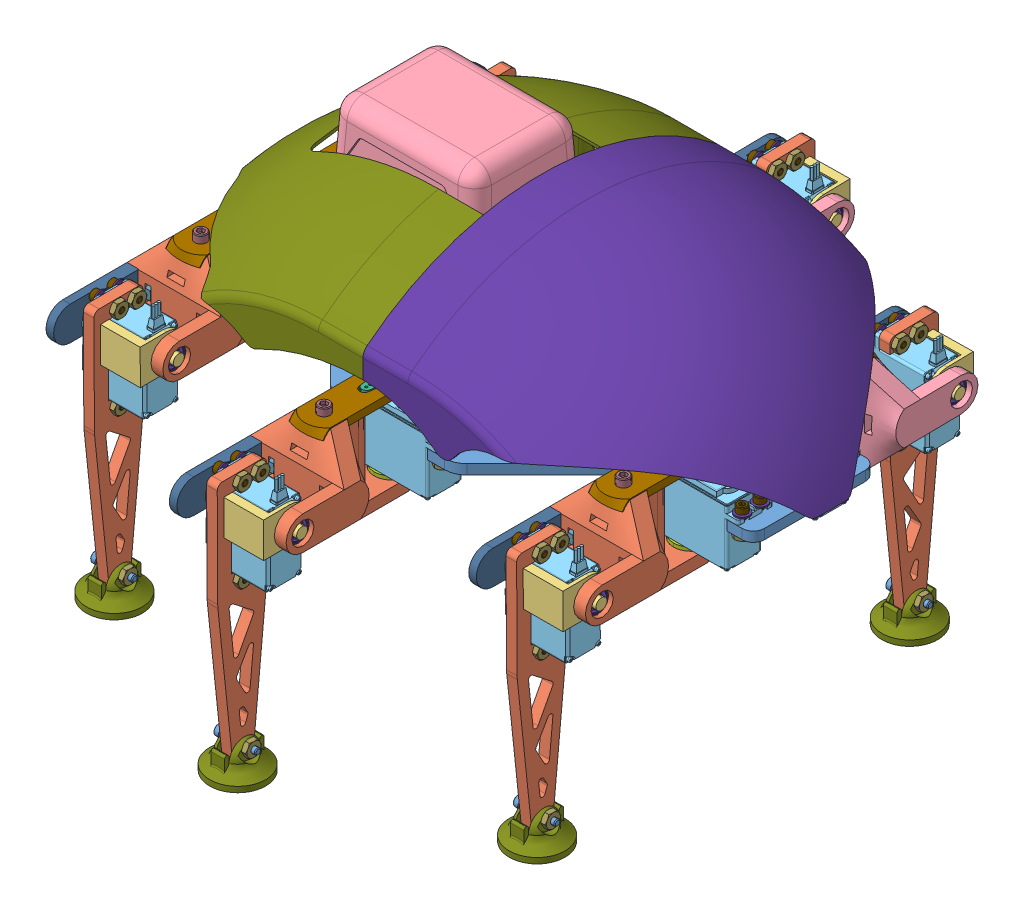
SolidWorks assembly Hexapod, configuration Défaut. Lengths in mm.
Overall size (338.69 233.7 350.77).
393 component instances, 35 part files, 155 mates.
Components (placement in the parent):
- Body_(Small)-5: Body_(Small) [Default] at (-310 -5.6 15) x (1 0 0) z (0 1 0) size (310 170 5.6)
- Leg_(Straight_Foot)-6: Leg_(Straight_Foot) [Default] at (-54.94 -26.67 -0.094) size (71.21 162.26 125.97) (flexible)
  - Foot_(Straight)-1: Foot_(Straight) [Default] at (4.9357 4.6704 -91.3697) x (0.014203 -0.004273 0.99989) z (-0.999899 0 0.014203) size (28 145.4 6)
  - bearing_mount_foot-1: bearing_mount_foot [Default] at (4.8169 16.6442 -99.7278) x (-0.014203 0.004273 -0.99989) z (0.999899 0 -0.014203) size (25 20 29.5)
  - Joint-1: Joint [Défaut] at (35.768 26.4662 -54.7315) x (-0.014203 0 -0.999899) z (0 1 0) size (96.52 53.26 53.26)
  - hs-422-2: hs-422 [Défaut] at (5.1023 6.612 -77.4562) x (-0.014203 0.004273 -0.99989) z (0.000061 0.999991 0.004272) size (19.81 42.09 58.23)
  - hs-422-3: hs-422 [Défaut] at (19.939 20.701 -19.812) x (0 0 1) z (-1 0 0) size (19.81 42.09 58.23)
  - hs-422_horn_straight-1: hs-422_horn_straight [Default] at (-16.9088 16.9412 -87.0065) x (0.014203 0 0.999899) z (0 1 0) size (33.93 4.93 8.79)
  - hs-422_horn_straight-2: hs-422_horn_straight [Default] at (9.652 42.5743 -9.906) x (-0.014203 0 -0.999899) z (-0.999899 0 0.014203) size (33.93 4.93 8.79)
  - Bearing_mount_leg-1: Bearing_mount_leg [Default] at (9.652 21 2.594) x (0 0 1) z (0 -1 0) size (35 20 30)
  - Bearing-1: Bearing [Default] at (9.652 -6.7498 -9.906) x (0.84763 0 0.530588) z (-0.530588 0 0.84763) size (13.87 4.75 13.87)
  - Bearing-2: Bearing [Default] at (32.2403 16.9412 -87.7047) x (0.007588 -0.845349 0.534161) z (-0.012007 -0.534214 -0.845264) size (13.87 4.75 13.87)
  - Joint_attachment_leg-1: Joint_attachment_leg [Défaut] at (35.768 26.4662 -54.7315) x (-0.014203 0 -0.999899) z (0 1 0) size (74.32 19.07 4.32)
  - Joint_attachment_foot-1: Joint_attachment_foot [Défaut] at (35.768 26.4662 -54.7315) x (-0.014203 0 -0.999899) z (0 1 0) size (64.08 6.7 19.07)
  - SBHCSCREW 0.112-40x0.25-HX-N-2: SBHCSCREW 0.112-40x0.25-HX-N [SBHCSCREW 0.112-40x0.25-HX-N] at (-19.9057 16.9412 -86.964) x (0.999899 0 -0.014203) z (-0.007102 0.866025 -0.49995) size (7.85 5.41 5.41)
  - SBHCSCREW 0.112-40x0.25-HX-N-3: SBHCSCREW 0.112-40x0.25-HX-N [SBHCSCREW 0.112-40x0.25-HX-N] at (9.652 45.5715 -9.906) x (0 -1 0) z (0.87304 0 0.487649) size (7.85 5.41 5.41)
  - MSHXNUT 0.138-32-D-N-15: MSHXNUT 0.138-32-D-N [MSHXNUT 0.138-32-D-N] at (5.0634 -17.1179 -82.3793) x (0.012331 0.496295 0.868066) z (-0.999899 0 0.014203) size (7.92 9.15 2.9)
  - MSHXNUT 0.138-32-D-N-16: MSHXNUT 0.138-32-D-N [MSHXNUT 0.138-32-D-N] at (4.9191 -17.0756 -92.5381) x (-0.01227 0.503696 -0.863794) z (-0.999899 0 0.014203) size (7.92 9.15 2.9)
  - MSHXNUT 0.138-32-D-N-17: MSHXNUT 0.138-32-D-N [MSHXNUT 0.138-32-D-N] at (5.0662 30.3817 -82.1827) x (0.000061 0.999991 0.004272) z (-0.999899 0 0.014203) size (7.92 9.15 2.9)
  - MSHXNUT 0.138-32-D-N-18: MSHXNUT 0.138-32-D-N [MSHXNUT 0.138-32-D-N] at (4.9219 30.4239 -92.3416) x (0.000061 0.999991 0.004272) z (-0.999899 0 0.014203) size (7.92 9.15 2.9)
  - HX-SHCS 0.164-32x0.5x0.5-N-1: HX-SHCS 0.164-32x0.5x0.5-N [HX-SHCS 0.164-32x0.5x0.5-N] at (9.1052 47.8568 -48.4) x (0 -1 0) z (0.014203 0 0.999899) size (16.87 6.86 6.86)
  - HX-SHCS 0.164-32x0.5x0.5-N-2: HX-SHCS 0.164-32x0.5x0.5-N [HX-SHCS 0.164-32x0.5x0.5-N] at (-21.967 16.9412 -59.205) x (0.999899 0 -0.014203) z (0.014203 0 0.999899) size (16.87 6.86 6.86)
  - MSHXNUT 0.164-32-D-N-11: MSHXNUT 0.164-32-D-N [MSHXNUT 0.164-32-D-N] at (9.1052 33.127 -48.4) x (0.87304 0 0.487649) z (0 1 0) size (8.74 10.09 3.3)
  - MSHXNUT 0.164-32-D-N-12: MSHXNUT 0.164-32-D-N [MSHXNUT 0.164-32-D-N] at (-7.2387 16.9412 -59.4142) x (0.014203 0 0.999899) z (-0.999899 0 0.014203) size (8.74 10.09 3.3)
  - HX-SHCS 0.112-40x0.5x0.5-N-7: HX-SHCS 0.112-40x0.5x0.5-N [HX-SHCS 0.112-40x0.5x0.5-N] at (-4.0273 11.7063 -99.6232) x (0.999899 0 -0.014203) z (0.014203 -0.004273 0.99989) size (15.54 4.65 4.65)
  - HX-SHCS 0.112-40x0.5x0.5-N-8: HX-SHCS 0.112-40x0.5x0.5-N [HX-SHCS 0.112-40x0.5x0.5-N] at (-4.0267 21.7062 -99.5805) x (0.999899 0 -0.014203) z (-0.014203 0.004273 -0.99989) size (15.54 4.65 4.65)
  - Slipper-1: Slipper [Default] at (1.9296 -111.2294 -91.7731) x (0.999899 0 -0.014203) z (0.014203 0 0.999899) size (35.48 18.25 37.71)
  - Narrow FW 0.138-1: Narrow FW 0.138 [Narrow FW 0.138] at (-3.4475 30.3814 -82.0597) x (0.999899 0 -0.014203) z (0.014203 0 0.999899) size (0.81 7.92 7.92)
  - HX-SHCS 0.138-32x0.5x0.5-N-2: HX-SHCS 0.138-32x0.5x0.5-N [HX-SHCS 0.138-32x0.5x0.5-N] at (-8.0191 30.3814 -81.9948) x (0.999899 0 -0.014203) z (0.014203 0 0.999899) size (16.21 5.74 5.74)
  - Narrow FW 0.138-2: Narrow FW 0.138 [Narrow FW 0.138] at (-3.4504 -17.1182 -82.2627) x (0.999899 0 -0.014203) z (0.014203 0 0.999899) size (0.81 7.92 7.92)
  - Narrow FW 0.138-3: Narrow FW 0.138 [Narrow FW 0.138] at (-3.5919 30.4248 -92.2186) x (0.999899 0 -0.014203) z (0.014203 0 0.999899) size (0.81 7.92 7.92)
  - Narrow FW 0.138-4: Narrow FW 0.138 [Narrow FW 0.138] at (-3.5947 -17.0748 -92.4216) x (0.999899 0 -0.014203) z (0.014203 0 0.999899) size (0.81 7.92 7.92)
  - HX-SHCS 0.138-32x0.5x0.5-N-3: HX-SHCS 0.138-32x0.5x0.5-N [HX-SHCS 0.138-32x0.5x0.5-N] at (-8.022 -17.1182 -82.1977) x (0.999899 0 -0.014203) z (0.014203 0 0.999899) size (16.21 5.74 5.74)
  - HX-SHCS 0.138-32x0.5x0.5-N-4: HX-SHCS 0.138-32x0.5x0.5-N [HX-SHCS 0.138-32x0.5x0.5-N] at (-8.1634 30.4248 -92.1537) x (0.999899 0 -0.014203) z (0.014203 0 0.999899) size (16.21 5.74 5.74)
  - HX-SHCS 0.138-32x0.5x0.5-N-5: HX-SHCS 0.138-32x0.5x0.5-N [HX-SHCS 0.138-32x0.5x0.5-N] at (-8.1663 -17.0748 -92.3566) x (0.999899 0 -0.014203) z (0.014203 0 0.999899) size (16.21 5.74 5.74)
  - HX-SHCS 0.138-32x0.5x0.5-N-6: HX-SHCS 0.138-32x0.5x0.5-N [HX-SHCS 0.138-32x0.5x0.5-N] at (-3.81 33.7566 -14.986) x (0 -1 0) z (-0.55878 0 0.829316) size (16.21 5.74 5.74)
  - Narrow FW 0.138-5: Narrow FW 0.138 [Narrow FW 0.138] at (-3.81 29.1846 -14.986) x (0 -1 0) z (0.55878 0 -0.829316) size (0.81 7.92 7.92)
  - Narrow FW 0.138-6: Narrow FW 0.138 [Narrow FW 0.138] at (43.69 29.1846 -14.986) x (0 -1 0) z (0.55878 0 -0.829316) size (0.81 7.92 7.92)
  - Narrow FW 0.138-7: Narrow FW 0.138 [Narrow FW 0.138] at (-3.81 29.1846 -4.826) x (0 -1 0) z (0.55878 0 -0.829316) size (0.81 7.92 7.92)
  - Narrow FW 0.138-8: Narrow FW 0.138 [Narrow FW 0.138] at (43.69 29.1846 -4.826) x (0 -1 0) z (0.55878 0 -0.829316) size (0.81 7.92 7.92)
  - HX-SHCS 0.138-32x0.5x0.5-N-7: HX-SHCS 0.138-32x0.5x0.5-N [HX-SHCS 0.138-32x0.5x0.5-N] at (43.69 33.7566 -14.986) x (0 -1 0) z (-0.55878 0 0.829316) size (16.21 5.74 5.74)
  - HX-SHCS 0.138-32x0.5x0.5-N-8: HX-SHCS 0.138-32x0.5x0.5-N [HX-SHCS 0.138-32x0.5x0.5-N] at (-3.81 33.7566 -4.826) x (0 -1 0) z (-0.55878 0 0.829316) size (16.21 5.74 5.74)
  - HX-SHCS 0.138-32x0.5x0.5-N-9: HX-SHCS 0.138-32x0.5x0.5-N [HX-SHCS 0.138-32x0.5x0.5-N] at (43.69 33.7566 -4.826) x (0 -1 0) z (-0.55878 0 0.829316) size (16.21 5.74 5.74)
  - HX-SHCS 0.138-32x0.75x0.75-N-10: HX-SHCS 0.138-32x0.75x0.75-N [HX-SHCS 0.138-32x0.75x0.75-N] at (-8.9913 -99.7294 -91.618) x (0.999899 0 -0.014203) z (-0.012539 -0.46966 -0.882758) size (22.56 5.74 5.74)
  - Narrow FW 0.138-10: Narrow FW 0.138 [Narrow FW 0.138] at (-5.2324 -99.7294 -91.6714) x (-0.999899 0 0.014203) z (-0.011665 -0.570502 -0.821213) size (0.81 7.92 7.92)
  - MSHXNUT 0.138-32-D-N-19: MSHXNUT 0.138-32-D-N [MSHXNUT 0.138-32-D-N] at (8.279 -99.7294 -91.8633) x (0 1 0) z (-0.999899 0 0.014203) size (7.92 9.15 2.9)
- Leg_(Straight_Foot)-7: Leg_(Straight_Foot) [Default] at (-294.94 -26.67 -0.094) size (71.21 162.26 125.97) (flexible)
  - Foot_(Straight)-1: Foot_(Straight) [Default] at (4.9357 4.6704 -91.3697) x (0.014203 -0.004273 0.99989) z (-0.999899 0 0.014203) size (28 145.4 6)
  - bearing_mount_foot-1: bearing_mount_foot [Default] at (4.8169 16.6442 -99.7278) x (-0.014203 0.004273 -0.99989) z (0.999899 0 -0.014203) size (25 20 29.5)
  - Joint-1: Joint [Défaut] at (35.768 26.4662 -54.7315) x (-0.014203 0 -0.999899) z (0 1 0) size (96.52 53.26 53.26)
  - hs-422-2: hs-422 [Défaut] at (5.1023 6.612 -77.4562) x (-0.014203 0.004273 -0.99989) z (0.000061 0.999991 0.004272) size (19.81 42.09 58.23)
  - hs-422-3: hs-422 [Défaut] at (19.939 20.701 -19.812) x (0 0 1) z (-1 0 0) size (19.81 42.09 58.23)
  - hs-422_horn_straight-1: hs-422_horn_straight [Default] at (-16.9088 16.9412 -87.0065) x (0.014203 0 0.999899) z (0 1 0) size (33.93 4.93 8.79)
  - hs-422_horn_straight-2: hs-422_horn_straight [Default] at (9.652 42.5743 -9.906) x (-0.014203 0 -0.999899) z (-0.999899 0 0.014203) size (33.93 4.93 8.79)
  - Bearing_mount_leg-1: Bearing_mount_leg [Default] at (9.652 21 2.594) x (0 0 1) z (0 -1 0) size (35 20 30)
  - Bearing-1: Bearing [Default] at (9.652 -6.7498 -9.906) x (0.84763 0 0.530588) z (-0.530588 0 0.84763) size (13.87 4.75 13.87)
  - Bearing-2: Bearing [Default] at (32.2403 16.9412 -87.7047) x (0.007588 -0.845349 0.534161) z (-0.012007 -0.534214 -0.845264) size (13.87 4.75 13.87)
  - Joint_attachment_leg-1: Joint_attachment_leg [Défaut] at (35.768 26.4662 -54.7315) x (-0.014203 0 -0.999899) z (0 1 0) size (74.32 19.07 4.32)
  - Joint_attachment_foot-1: Joint_attachment_foot [Défaut] at (35.768 26.4662 -54.7315) x (-0.014203 0 -0.999899) z (0 1 0) size (64.08 6.7 19.07)
  - SBHCSCREW 0.112-40x0.25-HX-N-2: SBHCSCREW 0.112-40x0.25-HX-N [SBHCSCREW 0.112-40x0.25-HX-N] at (-19.9057 16.9412 -86.964) x (0.999899 0 -0.014203) z (-0.007102 0.866025 -0.49995) size (7.85 5.41 5.41)
  - SBHCSCREW 0.112-40x0.25-HX-N-3: SBHCSCREW 0.112-40x0.25-HX-N [SBHCSCREW 0.112-40x0.25-HX-N] at (9.652 45.5715 -9.906) x (0 -1 0) z (0.87304 0 0.487649) size (7.85 5.41 5.41)
  - MSHXNUT 0.138-32-D-N-15: MSHXNUT 0.138-32-D-N [MSHXNUT 0.138-32-D-N] at (5.0634 -17.1179 -82.3793) x (0.012331 0.496295 0.868066) z (-0.999899 0 0.014203) size (7.92 9.15 2.9)
  - MSHXNUT 0.138-32-D-N-16: MSHXNUT 0.138-32-D-N [MSHXNUT 0.138-32-D-N] at (4.9191 -17.0756 -92.5381) x (-0.01227 0.503696 -0.863794) z (-0.999899 0 0.014203) size (7.92 9.15 2.9)
  - MSHXNUT 0.138-32-D-N-17: MSHXNUT 0.138-32-D-N [MSHXNUT 0.138-32-D-N] at (5.0662 30.3817 -82.1827) x (0.000061 0.999991 0.004272) z (-0.999899 0 0.014203) size (7.92 9.15 2.9)
  - MSHXNUT 0.138-32-D-N-18: MSHXNUT 0.138-32-D-N [MSHXNUT 0.138-32-D-N] at (4.9219 30.4239 -92.3416) x (0.000061 0.999991 0.004272) z (-0.999899 0 0.014203) size (7.92 9.15 2.9)
  - HX-SHCS 0.164-32x0.5x0.5-N-1: HX-SHCS 0.164-32x0.5x0.5-N [HX-SHCS 0.164-32x0.5x0.5-N] at (9.1052 47.8568 -48.4) x (0 -1 0) z (0.014203 0 0.999899) size (16.87 6.86 6.86)
  - HX-SHCS 0.164-32x0.5x0.5-N-2: HX-SHCS 0.164-32x0.5x0.5-N [HX-SHCS 0.164-32x0.5x0.5-N] at (-21.967 16.9412 -59.205) x (0.999899 0 -0.014203) z (0.014203 0 0.999899) size (16.87 6.86 6.86)
  - MSHXNUT 0.164-32-D-N-11: MSHXNUT 0.164-32-D-N [MSHXNUT 0.164-32-D-N] at (9.1052 33.127 -48.4) x (0.87304 0 0.487649) z (0 1 0) size (8.74 10.09 3.3)
  - MSHXNUT 0.164-32-D-N-12: MSHXNUT 0.164-32-D-N [MSHXNUT 0.164-32-D-N] at (-7.2387 16.9412 -59.4142) x (0.014203 0 0.999899) z (-0.999899 0 0.014203) size (8.74 10.09 3.3)
  - HX-SHCS 0.112-40x0.5x0.5-N-7: HX-SHCS 0.112-40x0.5x0.5-N [HX-SHCS 0.112-40x0.5x0.5-N] at (-4.0273 11.7063 -99.6232) x (0.999899 0 -0.014203) z (0.014203 -0.004273 0.99989) size (15.54 4.65 4.65)
  - HX-SHCS 0.112-40x0.5x0.5-N-8: HX-SHCS 0.112-40x0.5x0.5-N [HX-SHCS 0.112-40x0.5x0.5-N] at (-4.0267 21.7062 -99.5805) x (0.999899 0 -0.014203) z (-0.014203 0.004273 -0.99989) size (15.54 4.65 4.65)
  - Slipper-1: Slipper [Default] at (1.9296 -111.2294 -91.7731) x (0.999899 0 -0.014203) z (0.014203 0 0.999899) size (35.48 18.25 37.71)
  - Narrow FW 0.138-1: Narrow FW 0.138 [Narrow FW 0.138] at (-3.4475 30.3814 -82.0597) x (0.999899 0 -0.014203) z (0.014203 0 0.999899) size (0.81 7.92 7.92)
  - HX-SHCS 0.138-32x0.5x0.5-N-2: HX-SHCS 0.138-32x0.5x0.5-N [HX-SHCS 0.138-32x0.5x0.5-N] at (-8.0191 30.3814 -81.9948) x (0.999899 0 -0.014203) z (0.014203 0 0.999899) size (16.21 5.74 5.74)
  - Narrow FW 0.138-2: Narrow FW 0.138 [Narrow FW 0.138] at (-3.4504 -17.1182 -82.2627) x (0.999899 0 -0.014203) z (0.014203 0 0.999899) size (0.81 7.92 7.92)
  - Narrow FW 0.138-3: Narrow FW 0.138 [Narrow FW 0.138] at (-3.5919 30.4248 -92.2186) x (0.999899 0 -0.014203) z (0.014203 0 0.999899) size (0.81 7.92 7.92)
  - Narrow FW 0.138-4: Narrow FW 0.138 [Narrow FW 0.138] at (-3.5947 -17.0748 -92.4216) x (0.999899 0 -0.014203) z (0.014203 0 0.999899) size (0.81 7.92 7.92)
  - HX-SHCS 0.138-32x0.5x0.5-N-3: HX-SHCS 0.138-32x0.5x0.5-N [HX-SHCS 0.138-32x0.5x0.5-N] at (-8.022 -17.1182 -82.1977) x (0.999899 0 -0.014203) z (0.014203 0 0.999899) size (16.21 5.74 5.74)
  - HX-SHCS 0.138-32x0.5x0.5-N-4: HX-SHCS 0.138-32x0.5x0.5-N [HX-SHCS 0.138-32x0.5x0.5-N] at (-8.1634 30.4248 -92.1537) x (0.999899 0 -0.014203) z (0.014203 0 0.999899) size (16.21 5.74 5.74)
  - HX-SHCS 0.138-32x0.5x0.5-N-5: HX-SHCS 0.138-32x0.5x0.5-N [HX-SHCS 0.138-32x0.5x0.5-N] at (-8.1663 -17.0748 -92.3566) x (0.999899 0 -0.014203) z (0.014203 0 0.999899) size (16.21 5.74 5.74)
  - HX-SHCS 0.138-32x0.5x0.5-N-6: HX-SHCS 0.138-32x0.5x0.5-N [HX-SHCS 0.138-32x0.5x0.5-N] at (-3.81 33.7566 -14.986) x (0 -1 0) z (-0.55878 0 0.829316) size (16.21 5.74 5.74)
  - Narrow FW 0.138-5: Narrow FW 0.138 [Narrow FW 0.138] at (-3.81 29.1846 -14.986) x (0 -1 0) z (0.55878 0 -0.829316) size (0.81 7.92 7.92)
  - Narrow FW 0.138-6: Narrow FW 0.138 [Narrow FW 0.138] at (43.69 29.1846 -14.986) x (0 -1 0) z (0.55878 0 -0.829316) size (0.81 7.92 7.92)
  - Narrow FW 0.138-7: Narrow FW 0.138 [Narrow FW 0.138] at (-3.81 29.1846 -4.826) x (0 -1 0) z (0.55878 0 -0.829316) size (0.81 7.92 7.92)
  - Narrow FW 0.138-8: Narrow FW 0.138 [Narrow FW 0.138] at (43.69 29.1846 -4.826) x (0 -1 0) z (0.55878 0 -0.829316) size (0.81 7.92 7.92)
  - HX-SHCS 0.138-32x0.5x0.5-N-7: HX-SHCS 0.138-32x0.5x0.5-N [HX-SHCS 0.138-32x0.5x0.5-N] at (43.69 33.7566 -14.986) x (0 -1 0) z (-0.55878 0 0.829316) size (16.21 5.74 5.74)
  - HX-SHCS 0.138-32x0.5x0.5-N-8: HX-SHCS 0.138-32x0.5x0.5-N [HX-SHCS 0.138-32x0.5x0.5-N] at (-3.81 33.7566 -4.826) x (0 -1 0) z (-0.55878 0 0.829316) size (16.21 5.74 5.74)
  - HX-SHCS 0.138-32x0.5x0.5-N-9: HX-SHCS 0.138-32x0.5x0.5-N [HX-SHCS 0.138-32x0.5x0.5-N] at (43.69 33.7566 -4.826) x (0 -1 0) z (-0.55878 0 0.829316) size (16.21 5.74 5.74)
  - HX-SHCS 0.138-32x0.75x0.75-N-10: HX-SHCS 0.138-32x0.75x0.75-N [HX-SHCS 0.138-32x0.75x0.75-N] at (-8.9913 -99.7294 -91.618) x (0.999899 0 -0.014203) z (-0.012539 -0.46966 -0.882758) size (22.56 5.74 5.74)
  - Narrow FW 0.138-10: Narrow FW 0.138 [Narrow FW 0.138] at (-5.2324 -99.7294 -91.6714) x (-0.999899 0 0.014203) z (-0.011665 -0.570502 -0.821213) size (0.81 7.92 7.92)
  - MSHXNUT 0.138-32-D-N-19: MSHXNUT 0.138-32-D-N [MSHXNUT 0.138-32-D-N] at (8.279 -99.7294 -91.8633) x (0 1 0) z (-0.999899 0 0.014203) size (7.92 9.15 2.9)
- Leg_(Straight_Foot)-8: Leg_(Straight_Foot) [Default] at (-174.94 -26.67 -50.094) size (71.21 162.26 125.97) (flexible)
  - Foot_(Straight)-1: Foot_(Straight) [Default] at (4.9357 4.6704 -91.3697) x (0.014203 -0.004273 0.99989) z (-0.999899 0 0.014203) size (28 145.4 6)
  - bearing_mount_foot-1: bearing_mount_foot [Default] at (4.8169 16.6442 -99.7278) x (-0.014203 0.004273 -0.99989) z (0.999899 0 -0.014203) size (25 20 29.5)
  - Joint-1: Joint [Défaut] at (35.768 26.4662 -54.7315) x (-0.014203 0 -0.999899) z (0 1 0) size (96.52 53.26 53.26)
  - hs-422-2: hs-422 [Défaut] at (5.1023 6.612 -77.4562) x (-0.014203 0.004273 -0.99989) z (0.000061 0.999991 0.004272) size (19.81 42.09 58.23)
  - hs-422-3: hs-422 [Défaut] at (19.939 20.701 -19.812) x (0 0 1) z (-1 0 0) size (19.81 42.09 58.23)
  - hs-422_horn_straight-1: hs-422_horn_straight [Default] at (-16.9088 16.9412 -87.0065) x (0.014203 0 0.999899) z (0 1 0) size (33.93 4.93 8.79)
  - hs-422_horn_straight-2: hs-422_horn_straight [Default] at (9.652 42.5743 -9.906) x (-0.014203 0 -0.999899) z (-0.999899 0 0.014203) size (33.93 4.93 8.79)
  - Bearing_mount_leg-1: Bearing_mount_leg [Default] at (9.652 21 2.594) x (0 0 1) z (0 -1 0) size (35 20 30)
  - Bearing-1: Bearing [Default] at (9.652 -6.7498 -9.906) x (0.84763 0 0.530588) z (-0.530588 0 0.84763) size (13.87 4.75 13.87)
  - Bearing-2: Bearing [Default] at (32.2403 16.9412 -87.7047) x (0.007588 -0.845349 0.534161) z (-0.012007 -0.534214 -0.845264) size (13.87 4.75 13.87)
  - Joint_attachment_leg-1: Joint_attachment_leg [Défaut] at (35.768 26.4662 -54.7315) x (-0.014203 0 -0.999899) z (0 1 0) size (74.32 19.07 4.32)
  - Joint_attachment_foot-1: Joint_attachment_foot [Défaut] at (35.768 26.4662 -54.7315) x (-0.014203 0 -0.999899) z (0 1 0) size (64.08 6.7 19.07)
  - SBHCSCREW 0.112-40x0.25-HX-N-2: SBHCSCREW 0.112-40x0.25-HX-N [SBHCSCREW 0.112-40x0.25-HX-N] at (-19.9057 16.9412 -86.964) x (0.999899 0 -0.014203) z (-0.007102 0.866025 -0.49995) size (7.85 5.41 5.41)
  - SBHCSCREW 0.112-40x0.25-HX-N-3: SBHCSCREW 0.112-40x0.25-HX-N [SBHCSCREW 0.112-40x0.25-HX-N] at (9.652 45.5715 -9.906) x (0 -1 0) z (0.87304 0 0.487649) size (7.85 5.41 5.41)
  - MSHXNUT 0.138-32-D-N-15: MSHXNUT 0.138-32-D-N [MSHXNUT 0.138-32-D-N] at (5.0634 -17.1179 -82.3793) x (0.012331 0.496295 0.868066) z (-0.999899 0 0.014203) size (7.92 9.15 2.9)
  - MSHXNUT 0.138-32-D-N-16: MSHXNUT 0.138-32-D-N [MSHXNUT 0.138-32-D-N] at (4.9191 -17.0756 -92.5381) x (-0.01227 0.503696 -0.863794) z (-0.999899 0 0.014203) size (7.92 9.15 2.9)
  - MSHXNUT 0.138-32-D-N-17: MSHXNUT 0.138-32-D-N [MSHXNUT 0.138-32-D-N] at (5.0662 30.3817 -82.1827) x (0.000061 0.999991 0.004272) z (-0.999899 0 0.014203) size (7.92 9.15 2.9)
  - MSHXNUT 0.138-32-D-N-18: MSHXNUT 0.138-32-D-N [MSHXNUT 0.138-32-D-N] at (4.9219 30.4239 -92.3416) x (0.000061 0.999991 0.004272) z (-0.999899 0 0.014203) size (7.92 9.15 2.9)
  - HX-SHCS 0.164-32x0.5x0.5-N-1: HX-SHCS 0.164-32x0.5x0.5-N [HX-SHCS 0.164-32x0.5x0.5-N] at (9.1052 47.8568 -48.4) x (0 -1 0) z (0.014203 0 0.999899) size (16.87 6.86 6.86)
  - HX-SHCS 0.164-32x0.5x0.5-N-2: HX-SHCS 0.164-32x0.5x0.5-N [HX-SHCS 0.164-32x0.5x0.5-N] at (-21.967 16.9412 -59.205) x (0.999899 0 -0.014203) z (0.014203 0 0.999899) size (16.87 6.86 6.86)
  - MSHXNUT 0.164-32-D-N-11: MSHXNUT 0.164-32-D-N [MSHXNUT 0.164-32-D-N] at (9.1052 33.127 -48.4) x (0.87304 0 0.487649) z (0 1 0) size (8.74 10.09 3.3)
  - MSHXNUT 0.164-32-D-N-12: MSHXNUT 0.164-32-D-N [MSHXNUT 0.164-32-D-N] at (-7.2387 16.9412 -59.4142) x (0.014203 0 0.999899) z (-0.999899 0 0.014203) size (8.74 10.09 3.3)
  - HX-SHCS 0.112-40x0.5x0.5-N-7: HX-SHCS 0.112-40x0.5x0.5-N [HX-SHCS 0.112-40x0.5x0.5-N] at (-4.0273 11.7063 -99.6232) x (0.999899 0 -0.014203) z (0.014203 -0.004273 0.99989) size (15.54 4.65 4.65)
  - HX-SHCS 0.112-40x0.5x0.5-N-8: HX-SHCS 0.112-40x0.5x0.5-N [HX-SHCS 0.112-40x0.5x0.5-N] at (-4.0267 21.7062 -99.5805) x (0.999899 0 -0.014203) z (-0.014203 0.004273 -0.99989) size (15.54 4.65 4.65)
  - Slipper-1: Slipper [Default] at (1.9296 -111.2294 -91.7731) x (0.999899 0 -0.014203) z (0.014203 0 0.999899) size (35.48 18.25 37.71)
  - Narrow FW 0.138-1: Narrow FW 0.138 [Narrow FW 0.138] at (-3.4475 30.3814 -82.0597) x (0.999899 0 -0.014203) z (0.014203 0 0.999899) size (0.81 7.92 7.92)
  - HX-SHCS 0.138-32x0.5x0.5-N-2: HX-SHCS 0.138-32x0.5x0.5-N [HX-SHCS 0.138-32x0.5x0.5-N] at (-8.0191 30.3814 -81.9948) x (0.999899 0 -0.014203) z (0.014203 0 0.999899) size (16.21 5.74 5.74)
  - Narrow FW 0.138-2: Narrow FW 0.138 [Narrow FW 0.138] at (-3.4504 -17.1182 -82.2627) x (0.999899 0 -0.014203) z (0.014203 0 0.999899) size (0.81 7.92 7.92)
  - Narrow FW 0.138-3: Narrow FW 0.138 [Narrow FW 0.138] at (-3.5919 30.4248 -92.2186) x (0.999899 0 -0.014203) z (0.014203 0 0.999899) size (0.81 7.92 7.92)
  - Narrow FW 0.138-4: Narrow FW 0.138 [Narrow FW 0.138] at (-3.5947 -17.0748 -92.4216) x (0.999899 0 -0.014203) z (0.014203 0 0.999899) size (0.81 7.92 7.92)
  - HX-SHCS 0.138-32x0.5x0.5-N-3: HX-SHCS 0.138-32x0.5x0.5-N [HX-SHCS 0.138-32x0.5x0.5-N] at (-8.022 -17.1182 -82.1977) x (0.999899 0 -0.014203) z (0.014203 0 0.999899) size (16.21 5.74 5.74)
  - HX-SHCS 0.138-32x0.5x0.5-N-4: HX-SHCS 0.138-32x0.5x0.5-N [HX-SHCS 0.138-32x0.5x0.5-N] at (-8.1634 30.4248 -92.1537) x (0.999899 0 -0.014203) z (0.014203 0 0.999899) size (16.21 5.74 5.74)
  - HX-SHCS 0.138-32x0.5x0.5-N-5: HX-SHCS 0.138-32x0.5x0.5-N [HX-SHCS 0.138-32x0.5x0.5-N] at (-8.1663 -17.0748 -92.3566) x (0.999899 0 -0.014203) z (0.014203 0 0.999899) size (16.21 5.74 5.74)
  - HX-SHCS 0.138-32x0.5x0.5-N-6: HX-SHCS 0.138-32x0.5x0.5-N [HX-SHCS 0.138-32x0.5x0.5-N] at (-3.81 33.7566 -14.986) x (0 -1 0) z (-0.55878 0 0.829316) size (16.21 5.74 5.74)
  - Narrow FW 0.138-5: Narrow FW 0.138 [Narrow FW 0.138] at (-3.81 29.1846 -14.986) x (0 -1 0) z (0.55878 0 -0.829316) size (0.81 7.92 7.92)
  - Narrow FW 0.138-6: Narrow FW 0.138 [Narrow FW 0.138] at (43.69 29.1846 -14.986) x (0 -1 0) z (0.55878 0 -0.829316) size (0.81 7.92 7.92)
  - Narrow FW 0.138-7: Narrow FW 0.138 [Narrow FW 0.138] at (-3.81 29.1846 -4.826) x (0 -1 0) z (0.55878 0 -0.829316) size (0.81 7.92 7.92)
  - Narrow FW 0.138-8: Narrow FW 0.138 [Narrow FW 0.138] at (43.69 29.1846 -4.826) x (0 -1 0) z (0.55878 0 -0.829316) size (0.81 7.92 7.92)
  - HX-SHCS 0.138-32x0.5x0.5-N-7: HX-SHCS 0.138-32x0.5x0.5-N [HX-SHCS 0.138-32x0.5x0.5-N] at (43.69 33.7566 -14.986) x (0 -1 0) z (-0.55878 0 0.829316) size (16.21 5.74 5.74)
  - HX-SHCS 0.138-32x0.5x0.5-N-8: HX-SHCS 0.138-32x0.5x0.5-N [HX-SHCS 0.138-32x0.5x0.5-N] at (-3.81 33.7566 -4.826) x (0 -1 0) z (-0.55878 0 0.829316) size (16.21 5.74 5.74)
  - HX-SHCS 0.138-32x0.5x0.5-N-9: HX-SHCS 0.138-32x0.5x0.5-N [HX-SHCS 0.138-32x0.5x0.5-N] at (43.69 33.7566 -4.826) x (0 -1 0) z (-0.55878 0 0.829316) size (16.21 5.74 5.74)
  - HX-SHCS 0.138-32x0.75x0.75-N-10: HX-SHCS 0.138-32x0.75x0.75-N [HX-SHCS 0.138-32x0.75x0.75-N] at (-8.9913 -99.7294 -91.618) x (0.999899 0 -0.014203) z (-0.012539 -0.46966 -0.882758) size (22.56 5.74 5.74)
  - Narrow FW 0.138-10: Narrow FW 0.138 [Narrow FW 0.138] at (-5.2324 -99.7294 -91.6714) x (-0.999899 0 0.014203) z (-0.011665 -0.570502 -0.821213) size (0.81 7.92 7.92)
  - MSHXNUT 0.138-32-D-N-19: MSHXNUT 0.138-32-D-N [MSHXNUT 0.138-32-D-N] at (8.279 -99.7294 -91.8633) x (0 1 0) z (-0.999899 0 0.014203) size (7.92 9.15 2.9)
- Leg_(Straight_Foot)_(Mirror)-4: Leg_(Straight_Foot)_(Mirror) [Default] at (-294.94 -26.67 49.906) size (70.36 162.3 124.8) (flexible)
  - Joint_(Mirror)-1: Joint_(Mirror) [Défaut] at (36.4933 -51.1276 34.4889) x (0.002055 0 0.999998) z (0 -1 0) size (96.52 53.26 53.26)
  - hs-422-3: hs-422 [Défaut] at (19.939 20.701 -19.812) x (0 0 1) z (-1 0 0) size (19.81 42.09 58.23)
  - hs-422_horn_straight-2: hs-422_horn_straight [Default] at (9.652 42.5743 -9.906) x (0.002055 0 0.999998) z (0.999998 0 -0.002055) size (33.93 4.93 8.79)
  - Bearing_mount_leg-1: Bearing_mount_leg [Default] at (9.652 21 -22.406) x (0 0 -1) z (0 -1 0) size (35 20 30)
  - Bearing-1: Bearing [Default] at (9.652 -6.7498 -9.906) x (0.266287 0 0.963894) z (-0.963894 0 0.266287) size (13.87 4.75 13.87)
  - Joint_attachment_leg-1: Joint_attachment_leg [Défaut] at (-17.0066 26.5024 34.5989) x (0.002055 0 0.999998) z (0 1 0) size (74.32 19.07 4.32)
  - bearing_mount_foot-2: bearing_mount_foot [Default] at (6.7141 17.2663 79.9818) x (0.002055 -0.004919 0.999986) z (0.999998 0 -0.002055) size (25 20 29.5)
  - Bearing-3: Bearing [Default] at (29.1886 16.9774 67.524) x (-0.001098 -0.845349 -0.534213) z (0.001738 -0.534214 0.845347) size (13.87 4.75 13.87)
  - hs-422-4: hs-422 [Défaut] at (6.0779 6.6418 77.4268) x (-0.002055 0.004919 -0.999986) z (0.00001 0.999988 0.004919) size (19.81 42.09 58.23)
  - hs-422_horn_straight-3: hs-422_horn_straight [Default] at (-15.8156 16.9774 67.6165) x (-0.002055 0 -0.999998) z (0 -1 0) size (33.93 4.93 8.79)
  - Foot_(Straight)-2: Foot_(Straight) [Default] at (0.0967 4.6719 71.5233) x (-0.002055 0.004919 -0.999986) z (0.999998 0 -0.002055) size (28 145.4 6)
  - Joint_attachment_foot-2: Joint_attachment_foot [Défaut] at (36.4933 7.4524 34.4889) x (0.002055 0 0.999998) z (0 -1 0) size (64.08 6.7 19.07)
  - SBHCSCREW 0.138-32x0.25-HX-N-1: SBHCSCREW 0.138-32x0.25-HX-N [SBHCSCREW 0.138-32x0.25-HX-N] at (-19.1684 16.9774 67.6234) x (0.999998 0 -0.002055) z (0.002055 0 0.999998) size (8.2 6.65 6.65)
  - SBHCSCREW 0.138-32x0.25-HX-N-2: SBHCSCREW 0.138-32x0.25-HX-N [SBHCSCREW 0.138-32x0.25-HX-N] at (9.652 45.9271 -9.906) x (0 -1 0) z (-0.864996 0 0.501779) size (8.2 6.65 6.65)
  - HX-SHCS 0.112-40x0.5x0.5-N-5: HX-SHCS 0.112-40x0.5x0.5-N [HX-SHCS 0.112-40x0.5x0.5-N] at (-2.7306 21.6303 80.0227) x (0.999998 0 -0.002055) z (0.001019 -0.868474 0.495733) size (15.54 4.65 4.65)
  - HX-SHCS 0.112-40x0.5x0.5-N-6: HX-SHCS 0.112-40x0.5x0.5-N [HX-SHCS 0.112-40x0.5x0.5-N] at (-2.7307 11.6304 79.9735) x (0.999998 0 -0.002055) z (0.001036 0.863555 0.504253) size (15.54 4.65 4.65)
  - HX-SHCS 0.164-32x0.5x0.5-N-3: HX-SHCS 0.164-32x0.5x0.5-N [HX-SHCS 0.164-32x0.5x0.5-N] at (-21.1613 16.9774 39.9006) x (0.999998 0 -0.002055) z (0.001028 0.866025 0.499999) size (16.87 6.86 6.86)
  - HX-SHCS 0.164-32x0.5x0.5-N-4: HX-SHCS 0.164-32x0.5x0.5-N [HX-SHCS 0.164-32x0.5x0.5-N] at (9.7311 47.893 28.5918) x (0 -1 0) z (0.002055 0 0.999998) size (16.87 6.86 6.86)
  - MSHXNUT 0.138-32-D-N-14: MSHXNUT 0.138-32-D-N [MSHXNUT 0.138-32-D-N] at (6.0779 -17.0332 62.3241) x (-0.001785 -0.495734 -0.868473) z (-0.999998 0 0.002055) size (7.92 9.15 2.9)
  - MSHXNUT 0.138-32-D-N-15: MSHXNUT 0.138-32-D-N [MSHXNUT 0.138-32-D-N] at (8.9943 -17.0832 72.478) x (-0.001775 0.504254 -0.863554) z (0.999998 0 -0.002055) size (7.92 9.15 2.9)
  - MSHXNUT 0.138-32-D-N-16: MSHXNUT 0.138-32-D-N [MSHXNUT 0.138-32-D-N] at (8.9739 30.4662 62.5518) x (0.00001 0.999988 0.004919) z (0.999998 0 -0.002055) size (7.92 9.15 2.9)
  - MSHXNUT 0.138-32-D-N-17: MSHXNUT 0.138-32-D-N [MSHXNUT 0.138-32-D-N] at (6.0992 30.4162 72.7176) x (-0.001785 -0.495734 -0.868473) z (-0.999998 0 0.002055) size (7.92 9.15 2.9)
  - MSHXNUT 0.164-32-D-N-10: MSHXNUT 0.164-32-D-N [MSHXNUT 0.164-32-D-N] at (-6.4315 16.9774 39.8703) x (0.002055 0 0.999998) z (-0.999998 0 0.002055) size (8.74 10.09 3.3)
  - MSHXNUT 0.164-32-D-N-11: MSHXNUT 0.164-32-D-N [MSHXNUT 0.164-32-D-N] at (9.7311 29.8612 28.5918) x (-0.002055 0 -0.999998) z (0 -1 0) size (8.74 10.09 3.3)
  - Slipper-1: Slipper [Default] at (3.0957 -111.2276 71.0036) x (0.999998 0 -0.002055) z (0.002055 0 0.999998) size (35.48 18.25 37.71)
  - Narrow FW 0.138-4: Narrow FW 0.138 [Narrow FW 0.138] at (-2.4363 30.4642 62.5753) x (0.999998 0 -0.002055) z (0.002055 0 0.999998) size (0.81 7.92 7.92)
  - HX-SHCS 0.138-32x0.5x0.5-N-14: HX-SHCS 0.138-32x0.5x0.5-N [HX-SHCS 0.138-32x0.5x0.5-N] at (-7.0082 30.4642 62.5847) x (0.999998 0 -0.002055) z (0.002055 0 0.999998) size (16.21 5.74 5.74)
  - Narrow FW 0.138-5: Narrow FW 0.138 [Narrow FW 0.138] at (-2.4367 -17.0352 62.3416) x (0.999998 0 -0.002055) z (0.002055 0 0.999998) size (0.81 7.92 7.92)
  - Narrow FW 0.138-6: Narrow FW 0.138 [Narrow FW 0.138] at (-2.4154 30.4142 72.7351) x (0.999998 0 -0.002055) z (0.002055 0 0.999998) size (0.81 7.92 7.92)
  - Narrow FW 0.138-7: Narrow FW 0.138 [Narrow FW 0.138] at (-2.4158 -17.0852 72.5015) x (0.999998 0 -0.002055) z (0.002055 0 0.999998) size (0.81 7.92 7.92)
  - HX-SHCS 0.138-32x0.5x0.5-N-15: HX-SHCS 0.138-32x0.5x0.5-N [HX-SHCS 0.138-32x0.5x0.5-N] at (-7.0087 -17.0352 62.351) x (0.999998 0 -0.002055) z (0.002055 0 0.999998) size (16.21 5.74 5.74)
  - HX-SHCS 0.138-32x0.5x0.5-N-16: HX-SHCS 0.138-32x0.5x0.5-N [HX-SHCS 0.138-32x0.5x0.5-N] at (-6.9874 30.4142 72.7445) x (0.999998 0 -0.002055) z (0.002055 0 0.999998) size (16.21 5.74 5.74)
  - HX-SHCS 0.138-32x0.5x0.5-N-17: HX-SHCS 0.138-32x0.5x0.5-N [HX-SHCS 0.138-32x0.5x0.5-N] at (-6.9878 -17.0852 72.5109) x (0.999998 0 -0.002055) z (0.002055 0 0.999998) size (16.21 5.74 5.74)
  - Narrow FW 0.138-8: Narrow FW 0.138 [Narrow FW 0.138] at (-3.81 29.1846 -4.826) x (0 -1 0) z (0.55878 0 -0.829316) size (0.81 7.92 7.92)
  - HX-SHCS 0.138-32x0.5x0.5-N-18: HX-SHCS 0.138-32x0.5x0.5-N [HX-SHCS 0.138-32x0.5x0.5-N] at (-3.81 33.7566 -4.826) x (0 -1 0) z (-0.55878 0 0.829316) size (16.21 5.74 5.74)
  - Narrow FW 0.138-9: Narrow FW 0.138 [Narrow FW 0.138] at (43.69 29.1846 -4.826) x (0 -1 0) z (0.55878 0 -0.829316) size (0.81 7.92 7.92)
  - Narrow FW 0.138-10: Narrow FW 0.138 [Narrow FW 0.138] at (-3.81 29.1846 -14.986) x (0 -1 0) z (0.55878 0 -0.829316) size (0.81 7.92 7.92)
  - Narrow FW 0.138-11: Narrow FW 0.138 [Narrow FW 0.138] at (43.69 29.1846 -14.986) x (0 -1 0) z (0.55878 0 -0.829316) size (0.81 7.92 7.92)
  - HX-SHCS 0.138-32x0.5x0.5-N-19: HX-SHCS 0.138-32x0.5x0.5-N [HX-SHCS 0.138-32x0.5x0.5-N] at (43.69 33.7566 -4.826) x (0 -1 0) z (-0.55878 0 0.829316) size (16.21 5.74 5.74)
  - HX-SHCS 0.138-32x0.5x0.5-N-20: HX-SHCS 0.138-32x0.5x0.5-N [HX-SHCS 0.138-32x0.5x0.5-N] at (-3.81 33.7566 -14.986) x (0 -1 0) z (-0.55878 0 0.829316) size (16.21 5.74 5.74)
  - HX-SHCS 0.138-32x0.5x0.5-N-21: HX-SHCS 0.138-32x0.5x0.5-N [HX-SHCS 0.138-32x0.5x0.5-N] at (43.69 33.7566 -14.986) x (0 -1 0) z (-0.55878 0 0.829316) size (16.21 5.74 5.74)
  - HX-SHCS 0.138-32x0.75x0.75-N-1: HX-SHCS 0.138-32x0.75x0.75-N [HX-SHCS 0.138-32x0.75x0.75-N] at (-7.8263 -99.7276 71.0261) x (0.999998 0 -0.002055) z (-0.001815 -0.46966 -0.882845) size (22.56 5.74 5.74)
  - Narrow FW 0.138-12: Narrow FW 0.138 [Narrow FW 0.138] at (-4.0671 -99.7276 71.0183) x (-0.999998 0 0.002055) z (-0.001688 -0.570502 -0.821294) size (0.81 7.92 7.92)
  - MSHXNUT 0.138-32-D-N-18: MSHXNUT 0.138-32-D-N [MSHXNUT 0.138-32-D-N] at (9.4457 -99.7276 70.9906) x (0 1 0) z (-0.999998 0 0.002055) size (7.92 9.15 2.9)
- Leg_(Straight_Foot)_(Mirror)-5: Leg_(Straight_Foot)_(Mirror) [Default] at (-54.94 -26.67 49.906) size (70.36 162.3 124.8) (flexible)
  - Joint_(Mirror)-1: Joint_(Mirror) [Défaut] at (36.4933 -51.1276 34.4889) x (0.002055 0 0.999998) z (0 -1 0) size (96.52 53.26 53.26)
  - hs-422-3: hs-422 [Défaut] at (19.939 20.701 -19.812) x (0 0 1) z (-1 0 0) size (19.81 42.09 58.23)
  - hs-422_horn_straight-2: hs-422_horn_straight [Default] at (9.652 42.5743 -9.906) x (0.002055 0 0.999998) z (0.999998 0 -0.002055) size (33.93 4.93 8.79)
  - Bearing_mount_leg-1: Bearing_mount_leg [Default] at (9.652 21 -22.406) x (0 0 -1) z (0 -1 0) size (35 20 30)
  - Bearing-1: Bearing [Default] at (9.652 -6.7498 -9.906) x (0.266287 0 0.963894) z (-0.963894 0 0.266287) size (13.87 4.75 13.87)
  - Joint_attachment_leg-1: Joint_attachment_leg [Défaut] at (-17.0066 26.5024 34.5989) x (0.002055 0 0.999998) z (0 1 0) size (74.32 19.07 4.32)
  - bearing_mount_foot-2: bearing_mount_foot [Default] at (6.7141 17.2663 79.9818) x (0.002055 -0.004919 0.999986) z (0.999998 0 -0.002055) size (25 20 29.5)
  - Bearing-3: Bearing [Default] at (29.1886 16.9774 67.524) x (-0.001098 -0.845349 -0.534213) z (0.001738 -0.534214 0.845347) size (13.87 4.75 13.87)
  - hs-422-4: hs-422 [Défaut] at (6.0779 6.6418 77.4268) x (-0.002055 0.004919 -0.999986) z (0.00001 0.999988 0.004919) size (19.81 42.09 58.23)
  - hs-422_horn_straight-3: hs-422_horn_straight [Default] at (-15.8156 16.9774 67.6165) x (-0.002055 0 -0.999998) z (0 -1 0) size (33.93 4.93 8.79)
  - Foot_(Straight)-2: Foot_(Straight) [Default] at (0.0967 4.6719 71.5233) x (-0.002055 0.004919 -0.999986) z (0.999998 0 -0.002055) size (28 145.4 6)
  - Joint_attachment_foot-2: Joint_attachment_foot [Défaut] at (36.4933 7.4524 34.4889) x (0.002055 0 0.999998) z (0 -1 0) size (64.08 6.7 19.07)
  - SBHCSCREW 0.138-32x0.25-HX-N-1: SBHCSCREW 0.138-32x0.25-HX-N [SBHCSCREW 0.138-32x0.25-HX-N] at (-19.1684 16.9774 67.6234) x (0.999998 0 -0.002055) z (0.002055 0 0.999998) size (8.2 6.65 6.65)
  - SBHCSCREW 0.138-32x0.25-HX-N-2: SBHCSCREW 0.138-32x0.25-HX-N [SBHCSCREW 0.138-32x0.25-HX-N] at (9.652 45.9271 -9.906) x (0 -1 0) z (-0.864996 0 0.501779) size (8.2 6.65 6.65)
  - HX-SHCS 0.112-40x0.5x0.5-N-5: HX-SHCS 0.112-40x0.5x0.5-N [HX-SHCS 0.112-40x0.5x0.5-N] at (-2.7306 21.6303 80.0227) x (0.999998 0 -0.002055) z (0.001019 -0.868474 0.495733) size (15.54 4.65 4.65)
  - HX-SHCS 0.112-40x0.5x0.5-N-6: HX-SHCS 0.112-40x0.5x0.5-N [HX-SHCS 0.112-40x0.5x0.5-N] at (-2.7307 11.6304 79.9735) x (0.999998 0 -0.002055) z (0.001036 0.863555 0.504253) size (15.54 4.65 4.65)
  - HX-SHCS 0.164-32x0.5x0.5-N-3: HX-SHCS 0.164-32x0.5x0.5-N [HX-SHCS 0.164-32x0.5x0.5-N] at (-21.1613 16.9774 39.9006) x (0.999998 0 -0.002055) z (0.001028 0.866025 0.499999) size (16.87 6.86 6.86)
  - HX-SHCS 0.164-32x0.5x0.5-N-4: HX-SHCS 0.164-32x0.5x0.5-N [HX-SHCS 0.164-32x0.5x0.5-N] at (9.7311 47.893 28.5918) x (0 -1 0) z (0.002055 0 0.999998) size (16.87 6.86 6.86)
  - MSHXNUT 0.138-32-D-N-14: MSHXNUT 0.138-32-D-N [MSHXNUT 0.138-32-D-N] at (6.0779 -17.0332 62.3241) x (-0.001785 -0.495734 -0.868473) z (-0.999998 0 0.002055) size (7.92 9.15 2.9)
  - MSHXNUT 0.138-32-D-N-15: MSHXNUT 0.138-32-D-N [MSHXNUT 0.138-32-D-N] at (8.9943 -17.0832 72.478) x (-0.001775 0.504254 -0.863554) z (0.999998 0 -0.002055) size (7.92 9.15 2.9)
  - MSHXNUT 0.138-32-D-N-16: MSHXNUT 0.138-32-D-N [MSHXNUT 0.138-32-D-N] at (8.9739 30.4662 62.5518) x (0.00001 0.999988 0.004919) z (0.999998 0 -0.002055) size (7.92 9.15 2.9)
  - MSHXNUT 0.138-32-D-N-17: MSHXNUT 0.138-32-D-N [MSHXNUT 0.138-32-D-N] at (6.0992 30.4162 72.7176) x (-0.001785 -0.495734 -0.868473) z (-0.999998 0 0.002055) size (7.92 9.15 2.9)
  - MSHXNUT 0.164-32-D-N-10: MSHXNUT 0.164-32-D-N [MSHXNUT 0.164-32-D-N] at (-6.4315 16.9774 39.8703) x (0.002055 0 0.999998) z (-0.999998 0 0.002055) size (8.74 10.09 3.3)
  - MSHXNUT 0.164-32-D-N-11: MSHXNUT 0.164-32-D-N [MSHXNUT 0.164-32-D-N] at (9.7311 29.8612 28.5918) x (-0.002055 0 -0.999998) z (0 -1 0) size (8.74 10.09 3.3)
  - Slipper-1: Slipper [Default] at (3.0957 -111.2276 71.0036) x (0.999998 0 -0.002055) z (0.002055 0 0.999998) size (35.48 18.25 37.71)
  - Narrow FW 0.138-4: Narrow FW 0.138 [Narrow FW 0.138] at (-2.4363 30.4642 62.5753) x (0.999998 0 -0.002055) z (0.002055 0 0.999998) size (0.81 7.92 7.92)
  - HX-SHCS 0.138-32x0.5x0.5-N-14: HX-SHCS 0.138-32x0.5x0.5-N [HX-SHCS 0.138-32x0.5x0.5-N] at (-7.0082 30.4642 62.5847) x (0.999998 0 -0.002055) z (0.002055 0 0.999998) size (16.21 5.74 5.74)
  - Narrow FW 0.138-5: Narrow FW 0.138 [Narrow FW 0.138] at (-2.4367 -17.0352 62.3416) x (0.999998 0 -0.002055) z (0.002055 0 0.999998) size (0.81 7.92 7.92)
  - Narrow FW 0.138-6: Narrow FW 0.138 [Narrow FW 0.138] at (-2.4154 30.4142 72.7351) x (0.999998 0 -0.002055) z (0.002055 0 0.999998) size (0.81 7.92 7.92)
  - Narrow FW 0.138-7: Narrow FW 0.138 [Narrow FW 0.138] at (-2.4158 -17.0852 72.5015) x (0.999998 0 -0.002055) z (0.002055 0 0.999998) size (0.81 7.92 7.92)
